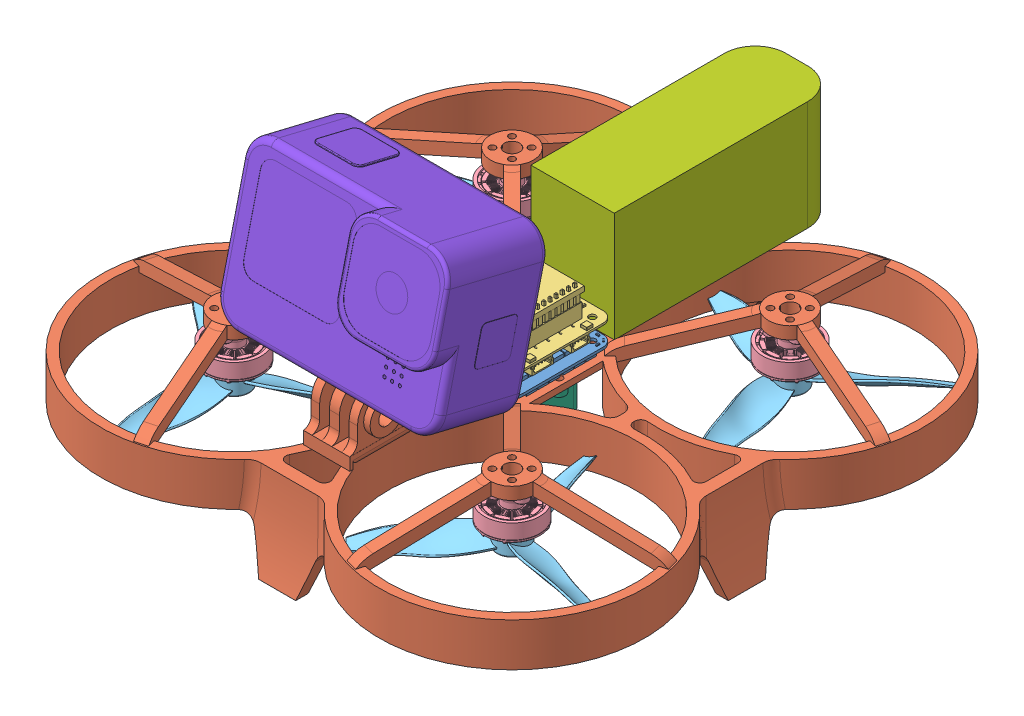
SolidWorks assembly Quad_assem, configuration Default. Lengths in mm.
Overall size (176 101.39 180.24).
14 component instances, 8 part files, 28 mates.
Components (placement in the parent):
- 4in1_ESC-1: 4in1_ESC [Default] at (-19 31.836 122.014) x (-1 0 0) z (0 1 0) size (33 33 7.6)
- Quad-1: Quad [Default] at (-19 0 122.014) x (-1 0 0) z (0 0 -1) size (176 48 176)
- FlightController.step-1: FlightController.step [Default] at (-19 38.5397 122.014) x (-1 0 0) z (0 1 0) size (33 33 15.78)
- 1404 motor.step-5: 1404 motor.step [Default] at (26 37 167.014) x (-0.963387 0 -0.268113) z (0 -1 0) size (17.9 17.9 14.53)
- Prop-1: Prop [Default] at (26 22.25 167.014) x (-0.291728 0 -0.956501) z (-0.956501 0 0.291728) size (58.53 5.95 67.58)
- Prop-2: Prop [Default] at (-64 22.25 167.014) x (-0.052615 0 0.998615) z (0.998615 0 0.052615) size (58.53 5.95 67.58)
- 1404 motor.step-6: 1404 motor.step [Default] at (-64 37 167.014) x (0.296226 0 0.955118) z (0 -1 0) size (17.9 17.9 14.53)
- Prop-3: Prop [Default] at (26 22.25 77.014) x (-0.951505 0 -0.307634) z (-0.307634 0 0.951505) size (58.53 5.95 67.58)
- 1404 motor.step-7: 1404 motor.step [Default] at (26 37 77.014) x (0.40894 0 -0.912561) z (0 -1 0) size (17.9 17.9 14.53)
- Prop-4: Prop [Default] at (-64 22.25 77.014) x (-0.967559 0 0.252646) z (0.252646 0 0.967559) size (58.53 5.95 67.58)
- 1404 motor.step-8: 1404 motor.step [Default] at (-64 37 77.014) x (0.79493 0 -0.606701) z (0 -1 0) size (17.9 17.9 14.53)
- ToF-1: ToF [Default] at (-19 27 122.014) x (1 0 0) z (0 0 -1) size (34.5 13.5 18.5)
- Battery-1: Battery [Default] at (-5.5403 46.75 66.0726) x (0 0 1) z (-1 0 0) size (72.6 35.5 27)
- GoPro Hero 9-1: GoPro Hero 9 [Default] at (-54.381 93.0618 145.1326) x (1 0 0) z (0 -0.97237 0.233445) size (72.1 33.6 50.5)
Mates (geometry in assembly coordinates):
- Concentric3: concentric aligned: circle of 4in1_ESC-1; circle of FlightController.step-1
- Concentric4: concentric aligned: circle of 4in1_ESC-1; circle of FlightController.step-1
- Distance3: distance = 6.08 mm anti-aligned: plane of 4in1_ESC-1 through (-2.5 31.836 109.014) normal (0 1 0); plane of FlightController.step-1 through (-2.5 37.916 109.014) normal (0 -1 0)
- Concentric5: concentric aligned: circle of 1404 motor.step-5; circle of Prop-1
- Concentric6: concentric aligned: circle of Prop-2; circle of 1404 motor.step-6
- Concentric7: concentric aligned: circle of Prop-3; circle of 1404 motor.step-7
- Concentric8: concentric aligned: circle of Prop-4; circle of 1404 motor.step-8
- Coincident17: coincident anti-aligned: plane of Prop-4 through (-64 25 77.014) normal (0 1 0); plane of 1404 motor.step-8 through (-64 25 77.014) normal (0 -1 0)
- Coincident18: coincident anti-aligned: plane of Prop-3 through (26 25 77.014) normal (0 1 0); plane of 1404 motor.step-7 through (26 25 77.014) normal (0 -1 0)
- Coincident19: coincident anti-aligned: plane of Prop-2 through (-64 25 167.014) normal (0 1 0); plane of 1404 motor.step-6 through (-64 25 167.014) normal (0 -1 0)
- Coincident20: coincident anti-aligned: plane of 1404 motor.step-5 through (26 25 167.014) normal (0 -1 0); plane of Prop-1 through (26 25 167.014) normal (0 1 0)
- Coincident21: coincident anti-aligned: plane of Quad-1 through (26 37 167.014) normal (0 -1 0); plane of 1404 motor.step-5 through (26 37 167.014) normal (0 1 0)
- Coincident22: coincident anti-aligned: plane of Quad-1 through (26 37 77.014) normal (0 -1 0); plane of 1404 motor.step-7 through (26 37 77.014) normal (0 1 0)
- Coincident23: coincident anti-aligned: plane of Quad-1 through (-64 37 77.014) normal (0 -1 0); plane of 1404 motor.step-8 through (-64 37 77.014) normal (0 1 0)
- Coincident24: coincident anti-aligned: plane of Quad-1 through (-64 37 167.014) normal (0 -1 0); plane of 1404 motor.step-6 through (-64 37 167.014) normal (0 1 0)
- Concentric9: concentric aligned: circle of Quad-1; circle of 1404 motor.step-7
- Concentric10: concentric aligned: circle of Quad-1; circle of 1404 motor.step-5
- Concentric11: concentric aligned: circle of Quad-1; circle of 1404 motor.step-6
- Concentric12: concentric aligned: circle of Quad-1; circle of 1404 motor.step-8
- Coincident27: coincident anti-aligned: plane of Quad-1 through (-4.5 27 107.514) normal (0 -1 0); plane of ToF-1 through (-8.3 27 115.264) normal (0 1 0)
- Concentric15: concentric anti-aligned: circle of Quad-1; circle of ToF-1
- Concentric16: concentric anti-aligned: circle of Quad-1; circle of ToF-1
- Concentric17: concentric aligned: circle of 4in1_ESC-1; circle of Quad-1
- Concentric18: concentric aligned: circle of Quad-1; circle of FlightController.step-1
- Coincident33: coincident anti-aligned: plane of 4in1_ESC-1 through (-2.5 31 109.014) normal (0 -1 0); plane of Quad-1 through (-6 31 135.014) normal (0 1 0)
- Coincident35: coincident anti-aligned: plane of Quad-1 through (-19 0 122.014) normal (0 -1 0)
- Coincident36: coincident anti-aligned: plane of Quad-1 through (-19 29 122.014) normal (0 1 0); plane of Battery-1 through (-32.5403 29 29.7726) normal (0 -1 0)
- Parallel1: parallel aligned: plane of Battery-1 through (-32.5403 29 102.3726) normal (0 0 1)
